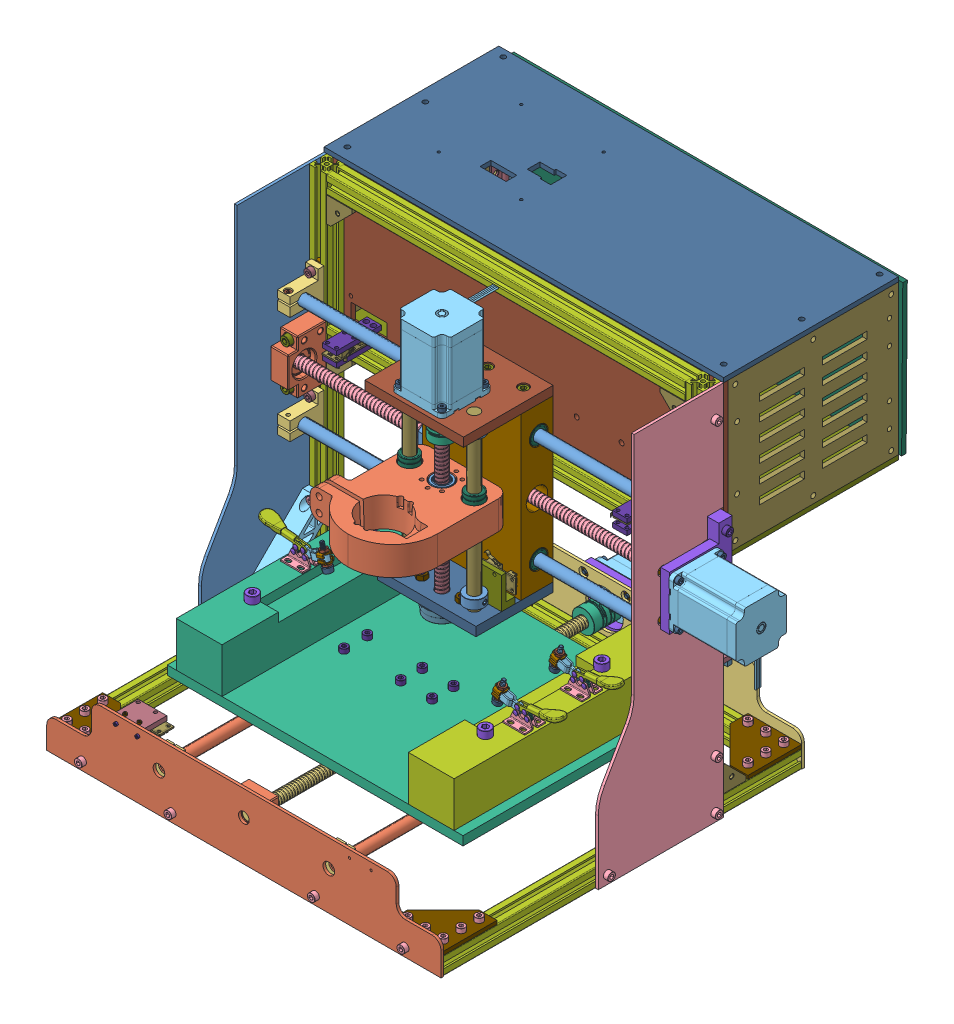
SolidWorks assembly CNC_DRILL1, configuration Default. Lengths in mm. (continued)
Components (placement in the parent): (continued)
- CUM_TAN_T-1: CUM_TAN_T [Default] at (66.2548 -100.7493 452.8517) x (-1 0 0) z (0 0 -1) size (20 34 34)
  - T-Nut_2020_M5.step-2-1: T-Nut_2020_M5.step-2 [Default] at (19.9061 6.5415 38.77) x (1 0 0) z (0 1 0) size (10 10.5 5)
  - T-Nut_2020_M5.step-2-2: T-Nut_2020_M5.step-2 [Default] at (19.9061 24.4415 20.87) size (10 10.5 5)
  - LBSBL6-2028-C_b-2-1: LBSBL6-2028-C_b-2 [Default] at (19.9061 8.5415 22.87) size (20 29.7 29.7)
- CUM_TAN_T-1-1: CUM_TAN_T-1 [Default] at (26.4425 -100.7493 427.1117) size (20 34 34)
  - T-Nut_2020_M5.step-2-1: T-Nut_2020_M5.step-2 [Default] at (19.9061 24.4415 20.87) size (10 10.5 5)
  - T-Nut_2020_M5.step-2-2: T-Nut_2020_M5.step-2 [Default] at (19.9061 6.5415 38.77) x (1 0 0) z (0 1 0) size (10 10.5 5)
  - LBSBL6-2028-C_b-2-1: LBSBL6-2028-C_b-2 [Default] at (19.9061 8.5415 22.87) size (20 29.7 29.7)
- CUM_TAN_T-2-1: CUM_TAN_T-2 [Default] at (486.2548 -100.7493 452.8517) x (-1 0 0) z (0 0 -1) size (20 34 34)
  - T-Nut_2020_M5.step-2-1: T-Nut_2020_M5.step-2 [Default] at (19.9061 24.4415 20.87) size (10 10.5 5)
  - T-Nut_2020_M5.step-2-2: T-Nut_2020_M5.step-2 [Default] at (19.9061 6.5415 38.77) x (1 0 0) z (0 1 0) size (10 10.5 5)
  - LBSBL6-2028-C_b-2-1: LBSBL6-2028-C_b-2 [Default] at (19.9061 8.5415 22.87) size (20 29.7 29.7)
- CUM_TAN_T-3-1: CUM_TAN_T-3 [Default] at (486.2548 -115.0778 441.4402) x (-1 0 0) z (0 1 0) size (20 34 34)
  - T-Nut_2020_M5.step-2-1: T-Nut_2020_M5.step-2 [Default] at (19.9061 24.4415 20.87) size (10 10.5 5)
  - T-Nut_2020_M5.step-2-2: T-Nut_2020_M5.step-2 [Default] at (19.9061 6.5415 38.77) x (1 0 0) z (0 1 0) size (10 10.5 5)
  - LBSBL6-2028-C_b-2-1: LBSBL6-2028-C_b-2 [Default] at (19.9061 8.5415 22.87) size (20 29.7 29.7)
- GH-201 (KECIL).STEP-1: GH-201 (KECIL).STEP [Default] at (384.0089 3.0167 494.044) size (81.05 32.54 23.05)
  - GH-201 (KECIL) PART 1.STEP-1: GH-201 (KECIL) PART 1.STEP [Default] at (0.3897 6.2755 23.667) size (24.52 11 10)
  - GH-201 (KECIL) PART 1.STEP-2: GH-201 (KECIL) PART 1.STEP [Default] at (24.8897 6.2755 0.6168) x (-1 0 0) z (0 0 -1) size (24.52 11 10)
  - GH-201 (KECIL) PART 2.STEP-1: GH-201 (KECIL) PART 2.STEP [Default] at (-14.4874 19.0399 16.1419) x (0.96092 -0.276826 0) z (0 0 1) size (28.48 12 8)
  - GH-201 (KECIL) PART 3.STEP-1: GH-201 (KECIL) PART 3.STEP [Default] at (16.2849 18.4306 12.167) x (0.434129 -0.900851 0) z (0 0 1) size (12 6 3)
  - GH-201 (KECIL) PART 4.STEP-1: GH-201 (KECIL) PART 4.STEP [Default] at (18.7026 25.6525 13.667) x (0.996652 0.081763 0) z (0 0 1) size (52.84 14.36 15)
  - GH-201 (KECIL) PIN.STEP-1: GH-201 (KECIL) PIN.STEP [Default] at (5.3978 13.1527 15.1668) x (0.991877 -0.127204 0) z (0 0 1) size (5 5 7.9)
  - GH-201 (KECIL) PIN.STEP-2: GH-201 (KECIL) PIN.STEP [Default] at (17.8978 13.1527 15.167) x (0.991877 -0.127204 0) z (0 0 1) size (5 5 7.9)
  - GH-201 (KECIL) PIN.STEP-3: GH-201 (KECIL) PIN.STEP [Default] at (7.1972 19.3987 15.1668) x (0.991877 -0.127204 0) z (0 0 1) size (5 5 7.9)
  - GH-201 (KECIL) PIN.STEP-4: GH-201 (KECIL) PIN.STEP [Default] at (15.2931 18.5578 15.1668) x (0.991877 -0.127204 0) z (0 0 1) size (5 5 7.9)
  - GH-201 (KECIL) CLIP.STEP-1: GH-201 (KECIL) CLIP.STEP [Default] at (-14.9027 17.5985 12.1419) x (-0.96092 0.276826 0) z (0 0 1) size (11 4 11)
  - GH-201 (KECIL) CLIP.STEP-2: GH-201 (KECIL) CLIP.STEP [Default] at (-12.1344 27.2077 12.1419) x (0.96092 -0.276826 0) z (0 0 1) size (11 4 11)
  - GH-201 (KECIL) PENEKAN.STEP-1: GH-201 (KECIL) PENEKAN.STEP [Default] at (-17.1675 9.7367 12.1419) x (0.942476 -0.271513 0.194986) z (-0.187366 0.053977 0.980806) size (10 27 10)
  - hex nut jam_am_B18.2.4.5M - Hex jam nut,  M5 x 0.8 --D-N.STEP-1: hex nut jam_am_B18.2.4.5M - Hex jam nut,  M5 x 0.8 --D-N.STEP [Default] at (-15.6501 15.0041 12.1419) x (0.96092 -0.276826 0) z (-0.276826 -0.96092 0) size (9.24 9.25 2.72)
  - hex nut jam_am_B18.2.4.5M - Hex jam nut,  M5 x 0.8 --D-N.STEP-2: hex nut jam_am_B18.2.4.5M - Hex jam nut,  M5 x 0.8 --D-N.STEP [Default] at (-11.387 29.8022 12.1419) x (0.96092 -0.276826 0) z (0.276826 0.96092 0) size (9.24 9.25 2.72)
- GH-201 (KECIL).STEP-1-1: GH-201 (KECIL).STEP-1 [Default] at (384.0089 3.0167 557.9937) size (81.05 32.54 23.05)
  - GH-201 (KECIL) PART 1.STEP-1: GH-201 (KECIL) PART 1.STEP [Default] at (24.8897 6.2755 0.6168) x (-1 0 0) z (0 0 -1) size (24.52 11 10)
  - GH-201 (KECIL) PART 1.STEP-2: GH-201 (KECIL) PART 1.STEP [Default] at (0.3897 6.2755 23.667) size (24.52 11 10)
  - GH-201 (KECIL) PART 2.STEP-1: GH-201 (KECIL) PART 2.STEP [Default] at (-14.4874 19.0399 16.1419) x (0.96092 -0.276826 0) z (0 0 1) size (28.48 12 8)
  - GH-201 (KECIL) PART 3.STEP-1: GH-201 (KECIL) PART 3.STEP [Default] at (16.2849 18.4306 12.167) x (0.434129 -0.900851 0) z (0 0 1) size (12 6 3)
  - GH-201 (KECIL) PART 4.STEP-1: GH-201 (KECIL) PART 4.STEP [Default] at (18.7026 25.6525 13.667) x (0.996652 0.081763 0) z (0 0 1) size (52.84 14.36 15)
  - GH-201 (KECIL) PIN.STEP-1: GH-201 (KECIL) PIN.STEP [Default] at (5.3978 13.1527 15.1668) x (0.991877 -0.127204 0) z (0 0 1) size (5 5 7.9)
  - GH-201 (KECIL) PIN.STEP-2: GH-201 (KECIL) PIN.STEP [Default] at (15.2931 18.5578 15.1668) x (0.991877 -0.127204 0) z (0 0 1) size (5 5 7.9)
  - GH-201 (KECIL) PIN.STEP-3: GH-201 (KECIL) PIN.STEP [Default] at (7.1972 19.3987 15.1668) x (0.991877 -0.127204 0) z (0 0 1) size (5 5 7.9)
  - GH-201 (KECIL) PIN.STEP-4: GH-201 (KECIL) PIN.STEP [Default] at (17.8978 13.1527 15.167) x (0.991877 -0.127204 0) z (0 0 1) size (5 5 7.9)
  - GH-201 (KECIL) CLIP.STEP-1: GH-201 (KECIL) CLIP.STEP [Default] at (-14.9027 17.5985 12.1419) x (-0.96092 0.276826 0) z (0 0 1) size (11 4 11)
  - GH-201 (KECIL) CLIP.STEP-2: GH-201 (KECIL) CLIP.STEP [Default] at (-12.1344 27.2077 12.1419) x (0.96092 -0.276826 0) z (0 0 1) size (11 4 11)
  - GH-201 (KECIL) PENEKAN.STEP-1: GH-201 (KECIL) PENEKAN.STEP [Default] at (-17.1675 9.7367 12.1419) x (0.942476 -0.271513 0.194986) z (-0.187366 0.053977 0.980806) size (10 27 10)
  - hex nut jam_am_B18.2.4.5M - Hex jam nut,  M5 x 0.8 --D-N.STEP-1: hex nut jam_am_B18.2.4.5M - Hex jam nut,  M5 x 0.8 --D-N.STEP [Default] at (-15.6501 15.0041 12.1419) x (0.96092 -0.276826 0) z (-0.276826 -0.96092 0) size (9.24 9.25 2.72)
  - hex nut jam_am_B18.2.4.5M - Hex jam nut,  M5 x 0.8 --D-N.STEP-2: hex nut jam_am_B18.2.4.5M - Hex jam nut,  M5 x 0.8 --D-N.STEP [Default] at (-11.387 29.8022 12.1419) x (0.96092 -0.276826 0) z (0.276826 0.96092 0) size (9.24 9.25 2.72)
- GH-201 (KECIL).STEP-2-1: GH-201 (KECIL).STEP-2 [Default] at (129.1884 3.0167 550.2775) x (-1 0 0) z (0 0 -1) size (81.05 32.54 23.05)
  - GH-201 (KECIL) PART 1.STEP-1: GH-201 (KECIL) PART 1.STEP [Default] at (0.3897 6.2755 23.667) size (24.52 11 10)
  - GH-201 (KECIL) PART 1.STEP-2: GH-201 (KECIL) PART 1.STEP [Default] at (24.8897 6.2755 0.6168) x (-1 0 0) z (0 0 -1) size (24.52 11 10)
  - GH-201 (KECIL) PART 2.STEP-1: GH-201 (KECIL) PART 2.STEP [Default] at (-14.4874 19.0399 16.1419) x (0.96092 -0.276826 0) z (0 0 1) size (28.48 12 8)
  - GH-201 (KECIL) PART 3.STEP-1: GH-201 (KECIL) PART 3.STEP [Default] at (16.2849 18.4306 12.167) x (0.434129 -0.900851 0) z (0 0 1) size (12 6 3)
  - GH-201 (KECIL) PART 4.STEP-1: GH-201 (KECIL) PART 4.STEP [Default] at (18.7026 25.6525 13.667) x (0.996652 0.081763 0) z (0 0 1) size (52.84 14.36 15)
  - GH-201 (KECIL) PIN.STEP-1: GH-201 (KECIL) PIN.STEP [Default] at (7.1972 19.3987 15.1668) x (0.991877 -0.127204 0) z (0 0 1) size (5 5 7.9)
  - GH-201 (KECIL) PIN.STEP-2: GH-201 (KECIL) PIN.STEP [Default] at (5.3978 13.1527 15.1668) x (0.991877 -0.127204 0) z (0 0 1) size (5 5 7.9)
  - GH-201 (KECIL) PIN.STEP-3: GH-201 (KECIL) PIN.STEP [Default] at (17.8978 13.1527 15.167) x (0.991877 -0.127204 0) z (0 0 1) size (5 5 7.9)
  - GH-201 (KECIL) PIN.STEP-4: GH-201 (KECIL) PIN.STEP [Default] at (15.2931 18.5578 15.1668) x (0.991877 -0.127204 0) z (0 0 1) size (5 5 7.9)
  - GH-201 (KECIL) CLIP.STEP-1: GH-201 (KECIL) CLIP.STEP [Default] at (-14.9027 17.5985 12.1419) x (-0.96092 0.276826 0) z (0 0 1) size (11 4 11)
  - GH-201 (KECIL) CLIP.STEP-2: GH-201 (KECIL) CLIP.STEP [Default] at (-12.1344 27.2077 12.1419) x (0.96092 -0.276826 0) z (0 0 1) size (11 4 11)
  - GH-201 (KECIL) PENEKAN.STEP-1: GH-201 (KECIL) PENEKAN.STEP [Default] at (-17.1675 9.7367 12.1419) x (0.942476 -0.271513 0.194986) z (-0.187366 0.053977 0.980806) size (10 27 10)
  - hex nut jam_am_B18.2.4.5M - Hex jam nut,  M5 x 0.8 --D-N.STEP-1: hex nut jam_am_B18.2.4.5M - Hex jam nut,  M5 x 0.8 --D-N.STEP [Default] at (-11.387 29.8022 12.1419) x (0.96092 -0.276826 0) z (0.276826 0.96092 0) size (9.24 9.25 2.72)
  - hex nut jam_am_B18.2.4.5M - Hex jam nut,  M5 x 0.8 --D-N.STEP-2: hex nut jam_am_B18.2.4.5M - Hex jam nut,  M5 x 0.8 --D-N.STEP [Default] at (-15.6501 15.0041 12.1419) x (0.96092 -0.276826 0) z (-0.276826 -0.96092 0) size (9.24 9.25 2.72)
- Assem1-1: Assem1 [Default] at (138.0975 -49.2059 785.2437) x (-1 0 0) z (0 0 -1) size (40.5 13.14 31.22)
  - Limit_switch-1: Limit_switch [Default] at (6.9988 2.8611 61.862) x (-1 0 0) z (0 0 -1) size (40.5 9 22.67)
  - Part101-1: Part101 [Default] at (11.2488 9.4981 60.262) x (1 0 0) z (0 -1 0) size (32 25 5)
  - Part15-1: Part15 [Default] at (11.2488 1.9981 45.262) size (32 5 5)
- Assem1-1-1: Assem1-1 [Default] at (371.0998 -49.2059 294.7198) size (40.5 13.14 31.22)
  - Limit_switch-1: Limit_switch [Default] at (6.9988 2.8611 61.862) x (-1 0 0) z (0 0 -1) size (40.5 9 22.67)
  - Part101-1: Part101 [Default] at (11.2488 9.4981 60.262) x (1 0 0) z (0 -1 0) size (32 25 5)
  - Part15-1: Part15 [Default] at (11.2488 1.9981 45.262) size (32 5 5)
- CONG_TAC_2-1: CONG_TAC_2 [Default] at (248.0157 229.2239 470.9282) x (-1 0 0) z (0 0 1) size (42.3 46.22 15)
  - Limit_switch-1: Limit_switch [Default] at (24.7058 33.7317 35.7236) x (1 0 0) z (0 -1 0) size (40.5 9 22.67)
  - 3D_IN_2-1: 3D_IN_2 [Default] at (18.6558 32.1317 36.4836) size (32 40 15)
- CONG_TAC_3-1: CONG_TAC_3 [Default] at (285.9024 40.7719 478.8031) size (42.3 41.22 15)
  - Limit_switch-1: Limit_switch [Default] at (20.0775 32.9203 29.9187) x (1 0 0) z (0 -1 0) size (40.5 9 22.67)
  - 3D_IN_3-1: 3D_IN_3 [Default] at (14.0275 31.3203 30.6787) size (32 35 15)
- Assem21-1: Assem21 [Default] at (134.1207 169.7573 469.2393) x (0 0 -1) z (-1 0 0) size (50.1 16.81 22.67)
  - Limit_switch-1: Limit_switch [Default] at (4.4076 3.2051 40.1721) size (40.5 9 22.67)
  - Part178-1: Part178 [Default] at (9.2576 3.9651 39.7721) size (50 5 16)
  - Part178-2: Part178 [Default] at (9.2576 -7.8449 39.7721) size (50 5 16)
- Assem21-1-1: Assem21-1 [Default] at (378.5766 168.6371 469.2393) x (0 0 -1) z (1 0 0) size (50.1 16.81 22.67)
  - Limit_switch-1: Limit_switch [Default] at (4.4076 3.2051 40.1721) size (40.5 9 22.67)
  - Part178-1: Part178 [Default] at (9.2576 3.9651 39.7721) size (50 5 16)
  - Part178-2: Part178 [Default] at (9.2576 -7.8449 39.7721) size (50 5 16)
- socket head cap screw_iso(ISO 4762 M5 x 8 - 8N)-1: socket head cap screw_iso(ISO 4762 M5 x 8 - 8N) [Default] at (66.3487 -83.2078 729.9817) x (0 -1 0) z (0 0 1) size (13 8.5 8.5)
- socket head cap screw_iso(ISO 4762 M5 x 8 - 8N)-2: socket head cap screw_iso(ISO 4762 M5 x 8 - 8N) [Default] at (446.3487 -83.2078 349.9817) x (0 -1 0) z (0 0 1) size (13 8.5 8.5)
- socket head cap screw_iso(ISO 4762 M5 x 8 - 8N)-3: socket head cap screw_iso(ISO 4762 M5 x 8 - 8N) [Default] at (46.3487 -83.2078 689.9817) x (0 -1 0) z (0 0 1) size (13 8.5 8.5)
- socket head cap screw_iso(ISO 4762 M5 x 8 - 8N)-4: socket head cap screw_iso(ISO 4762 M5 x 8 - 8N) [Default] at (46.3487 -83.2078 729.9817) x (0 -1 0) z (0 0 1) size (13 8.5 8.5)
- socket head cap screw_iso(ISO 4762 M5 x 8 - 8N)-5: socket head cap screw_iso(ISO 4762 M5 x 8 - 8N) [Default] at (28.3487 -102.2078 559.9817) size (13 8.5 8.5)
- socket head cap screw_iso(ISO 4762 M5 x 8 - 8N)-6: socket head cap screw_iso(ISO 4762 M5 x 8 - 8N) [Default] at (46.3487 -8.7078 458.9817) x (0 0 -1) z (1 0 0) size (13 8.5 8.5)
- socket head cap screw_iso(ISO 4762 M5 x 8 - 8N)-7: socket head cap screw_iso(ISO 4762 M5 x 8 - 8N) [Default] at (466.3487 -83.2078 729.9817) x (0 -1 0) z (0 0 1) size (13 8.5 8.5)
- socket head cap screw_iso(ISO 4762 M5 x 8 - 8N)-8: socket head cap screw_iso(ISO 4762 M5 x 8 - 8N) [Default] at (447.3487 -102.2078 439.9817) size (13 8.5 8.5)
- socket head cap screw_iso(ISO 4762 M5 x 8 - 8N)-9: socket head cap screw_iso(ISO 4762 M5 x 8 - 8N) [Default] at (466.3487 -83.2078 709.9817) x (0 -1 0) z (0 0 1) size (13 8.5 8.5)
- socket head cap screw_iso(ISO 4762 M5 x 8 - 8N)-10: socket head cap screw_iso(ISO 4762 M5 x 8 - 8N) [Default] at (336.3487 -102.2078 331.9817) x (0 0 1) z (-1 0 0) size (13 8.5 8.5)
- socket head cap screw_iso(ISO 4762 M5 x 8 - 8N)-11: socket head cap screw_iso(ISO 4762 M5 x 8 - 8N) [Default] at (65.3487 -62.2078 439.9817) x (-1 0 0) z (0 0.924225 0.381849) size (13 8.5 8.5)
- socket head cap screw_iso(ISO 4762 M5 x 8 - 8N)-12: socket head cap screw_iso(ISO 4762 M5 x 8 - 8N) [Default] at (466.3487 -83.2078 533.4817) x (0 -1 0) z (0 0 1) size (13 8.5 8.5)
- socket head cap screw_iso(ISO 4762 M5 x 8 - 8N)-13: socket head cap screw_iso(ISO 4762 M5 x 8 - 8N) [Default] at (436.8487 -102.2078 747.9817) x (0 0 -1) z (1 0 0) size (13 8.5 8.5)
- socket head cap screw_iso(ISO 4762 M5 x 8 - 8N)-14: socket head cap screw_iso(ISO 4762 M5 x 8 - 8N) [Default] at (46.3487 -83.2078 465.8817) x (0 -1 0) z (0.924225 0 -0.381849) size (13 8.5 8.5)
- socket head cap screw_iso(ISO 4762 M5 x 8 - 8N)-15: socket head cap screw_iso(ISO 4762 M5 x 8 - 8N) [Default] at (466.3487 -83.2078 369.9817) x (0 -1 0) z (0 0 1) size (13 8.5 8.5)
- socket head cap screw_iso(ISO 4762 M5 x 8 - 8N)-16: socket head cap screw_iso(ISO 4762 M5 x 8 - 8N) [Default] at (46.3487 -76.3078 458.9817) x (0 0 -1) z (0.381849 -0.924225 0) size (13 8.5 8.5)
- socket head cap screw_iso(ISO 4762 M5 x 8 - 8N)-17: socket head cap screw_iso(ISO 4762 M5 x 8 - 8N) [Default] at (484.3487 -47.2078 439.9817) x (-1 0 0) z (0 0.924225 0.381849) size (13 8.5 8.5)
- socket head cap screw_iso(ISO 4762 M5 x 8 - 8N)-18: socket head cap screw_iso(ISO 4762 M5 x 8 - 8N) [Default] at (176.3487 -102.2078 331.9817) x (0 0 1) z (-1 0 0) size (13 8.5 8.5)
- socket head cap screw_iso(ISO 4762 M5 x 8 - 8N)-19: socket head cap screw_iso(ISO 4762 M5 x 8 - 8N) [Default] at (466.3487 -83.2078 465.8817) x (0 -1 0) z (0.913871 0 -0.406005) size (13 8.5 8.5)
- socket head cap screw_iso(ISO 4762 M5 x 8 - 8N)-20: socket head cap screw_iso(ISO 4762 M5 x 8 - 8N) [Default] at (28.3487 77.7922 439.9817) size (13 8.5 8.5)
- socket head cap screw_iso(ISO 4762 M5 x 8 - 8N)-21: socket head cap screw_iso(ISO 4762 M5 x 8 - 8N) [Default] at (46.3487 -83.2078 414.0817) x (0 -1 0) z (0 0 1) size (13 8.5 8.5)
- socket head cap screw_iso(ISO 4762 M5 x 8 - 8N)-22: socket head cap screw_iso(ISO 4762 M5 x 8 - 8N) [Default] at (76.8487 -102.2078 747.9817) x (0 0 -1) z (1 0 0) size (13 8.5 8.5)
- socket head cap screw_iso(ISO 4762 M5 x 8 - 8N)-23: socket head cap screw_iso(ISO 4762 M5 x 8 - 8N) [Default] at (176.8487 -102.2078 747.9817) x (0 0 -1) z (1 0 0) size (13 8.5 8.5)
- socket head cap screw_iso(ISO 4762 M5 x 8 - 8N)-24: socket head cap screw_iso(ISO 4762 M5 x 8 - 8N) [Default] at (76.3487 -102.2078 331.9817) x (0 0 1) z (-1 0 0) size (13 8.5 8.5)
- socket head cap screw_iso(ISO 4762 M5 x 8 - 8N)-25: socket head cap screw_iso(ISO 4762 M5 x 8 - 8N) [Default] at (447.3487 -82.2078 439.9817) size (13 8.5 8.5)
- socket head cap screw_iso(ISO 4762 M5 x 8 - 8N)-26: socket head cap screw_iso(ISO 4762 M5 x 8 - 8N) [Default] at (65.3487 -82.2078 439.9817) x (-1 0 0) z (0 0.924225 0.381849) size (13 8.5 8.5)
- socket head cap screw_iso(ISO 4762 M5 x 8 - 8N)-27: socket head cap screw_iso(ISO 4762 M5 x 8 - 8N) [Default] at (446.3487 -83.2078 729.9817) x (0 -1 0) z (0 0 1) size (13 8.5 8.5)
- socket head cap screw_iso(ISO 4762 M5 x 8 - 8N)-28: socket head cap screw_iso(ISO 4762 M5 x 8 - 8N) [Default] at (447.3487 -102.2078 479.9817) size (13 8.5 8.5)
- socket head cap screw_iso(ISO 4762 M5 x 8 - 8N)-29: socket head cap screw_iso(ISO 4762 M5 x 8 - 8N) [Default] at (466.3487 -83.2078 689.9817) x (0 -1 0) z (0 0 1) size (13 8.5 8.5)
- socket head cap screw_iso(ISO 4762 M5 x 8 - 8N)-30: socket head cap screw_iso(ISO 4762 M5 x 8 - 8N) [Default] at (65.3487 -102.2078 459.9817) x (-1 0 0) z (0 0.924225 0.381849) size (13 8.5 8.5)
- socket head cap screw_iso(ISO 4762 M5 x 8 - 8N)-31: socket head cap screw_iso(ISO 4762 M5 x 8 - 8N) [Default] at (46.3487 -76.3078 420.9817) x (0 0 1) z (-0.565374 -0.824835 0) size (13 8.5 8.5)
- socket head cap screw_iso(ISO 4762 M5 x 8 - 8N)-32: socket head cap screw_iso(ISO 4762 M5 x 8 - 8N) [Default] at (466.3487 -83.2078 349.9817) x (0 -1 0) z (0 0 1) size (13 8.5 8.5)
- socket head cap screw_iso(ISO 4762 M5 x 8 - 8N)-33: socket head cap screw_iso(ISO 4762 M5 x 8 - 8N) [Default] at (65.3487 -102.2078 439.9817) x (-1 0 0) z (0 0.924225 0.381849) size (13 8.5 8.5)
- socket head cap screw_iso(ISO 4762 M5 x 8 - 8N)-34: socket head cap screw_iso(ISO 4762 M5 x 8 - 8N) [Default] at (466.3487 -83.2078 389.9817) x (0 -1 0) z (0 0 1) size (13 8.5 8.5)
- socket head cap screw_iso(ISO 4762 M5 x 8 - 8N)-35: socket head cap screw_iso(ISO 4762 M5 x 8 - 8N) [Default] at (484.3487 77.7922 439.9817) x (-1 0 0) z (0 0.924225 0.381849) size (13 8.5 8.5)
- socket head cap screw_iso(ISO 4762 M5 x 8 - 8N)-36: socket head cap screw_iso(ISO 4762 M5 x 8 - 8N) [Default] at (46.3487 -83.2078 533.4817) x (0 -1 0) z (0 0 1) size (13 8.5 8.5)
- socket head cap screw_iso(ISO 4762 M5 x 8 - 8N)-37: socket head cap screw_iso(ISO 4762 M5 x 8 - 8N) [Default] at (28.3487 -47.2078 439.9817) size (13 8.5 8.5)
- socket head cap screw_iso(ISO 4762 M5 x 8 - 8N)-38: socket head cap screw_iso(ISO 4762 M5 x 8 - 8N) [Default] at (66.3487 -83.2078 349.9817) x (0 -1 0) z (0 0 1) size (13 8.5 8.5)
- socket head cap screw_iso(ISO 4762 M5 x 8 - 8N)-39: socket head cap screw_iso(ISO 4762 M5 x 8 - 8N) [Default] at (426.3487 -83.2078 349.9817) x (0 -1 0) z (0 0 1) size (13 8.5 8.5)
- socket head cap screw_iso(ISO 4762 M5 x 8 - 8N)-40: socket head cap screw_iso(ISO 4762 M5 x 8 - 8N) [Default] at (86.3487 -83.2078 349.9817) x (0 -1 0) z (0 0 1) size (13 8.5 8.5)
- socket head cap screw_iso(ISO 4762 M5 x 8 - 8N)-41: socket head cap screw_iso(ISO 4762 M5 x 8 - 8N) [Default] at (46.3487 -83.2078 349.9817) x (0 -1 0) z (0 0 1) size (13 8.5 8.5)
- socket head cap screw_iso(ISO 4762 M5 x 8 - 8N)-42: socket head cap screw_iso(ISO 4762 M5 x 8 - 8N) [Default] at (426.3487 -83.2078 729.9817) x (0 -1 0) z (0 0 1) size (13 8.5 8.5)
- socket head cap screw_iso(ISO 4762 M5 x 8 - 8N)-43: socket head cap screw_iso(ISO 4762 M5 x 8 - 8N) [Default] at (28.3487 -102.2078 439.9817) size (13 8.5 8.5)
- socket head cap screw_iso(ISO 4762 M5 x 8 - 8N)-44: socket head cap screw_iso(ISO 4762 M5 x 8 - 8N) [Default] at (466.3487 -76.3078 458.9817) x (0 0 -1) z (0.994603 0.103758 0) size (13 8.5 8.5)
- socket head cap screw_iso(ISO 4762 M5 x 8 - 8N)-45: socket head cap screw_iso(ISO 4762 M5 x 8 - 8N) [Default] at (466.3487 -8.7078 458.9817) x (0 0 -1) z (1 0 0) size (13 8.5 8.5)
- socket head cap screw_iso(ISO 4762 M5 x 8 - 8N)-46: socket head cap screw_iso(ISO 4762 M5 x 8 - 8N) [Default] at (484.3487 -102.2078 439.9817) x (-1 0 0) z (0 0.924225 0.381849) size (13 8.5 8.5)
- socket head cap screw_iso(ISO 4762 M5 x 8 - 8N)-47: socket head cap screw_iso(ISO 4762 M5 x 8 - 8N) [Default] at (336.8487 -102.2078 747.9817) x (0 0 -1) z (1 0 0) size (13 8.5 8.5)
- socket head cap screw_iso(ISO 4762 M5 x 8 - 8N)-48: socket head cap screw_iso(ISO 4762 M5 x 8 - 8N) [Default] at (46.3487 -83.2078 709.9817) x (0 -1 0) z (0 0 1) size (13 8.5 8.5)
- socket head cap screw_iso(ISO 4762 M5 x 8 - 8N)-49: socket head cap screw_iso(ISO 4762 M5 x 8 - 8N) [Default] at (86.3487 -83.2078 729.9817) x (0 -1 0) z (0 0 1) size (13 8.5 8.5)
- socket head cap screw_iso(ISO 4762 M5 x 8 - 8N)-50: socket head cap screw_iso(ISO 4762 M5 x 8 - 8N) [Default] at (447.3487 -62.2078 439.9817) size (13 8.5 8.5)
- socket head cap screw_iso(ISO 4762 M5 x 8 - 8N)-51: socket head cap screw_iso(ISO 4762 M5 x 8 - 8N) [Default] at (436.3487 -102.2078 331.9817) x (0 0 1) z (-1 0 0) size (13 8.5 8.5)
- socket head cap screw_iso(ISO 4762 M5 x 8 - 8N)-52: socket head cap screw_iso(ISO 4762 M5 x 8 - 8N) [Default] at (484.3487 277.7922 439.9817) x (-1 0 0) z (0 0.924225 0.381849) size (13 8.5 8.5)
- socket head cap screw_iso(ISO 4762 M5 x 8 - 8N)-53: socket head cap screw_iso(ISO 4762 M5 x 8 - 8N) [Default] at (484.3487 -102.2078 559.9817) x (-1 0 0) z (0 0.924225 0.381849) size (13 8.5 8.5)
- socket head cap screw_iso(ISO 4762 M5 x 8 - 8N)-54: socket head cap screw_iso(ISO 4762 M5 x 8 - 8N) [Default] at (466.3487 -83.2078 414.0817) x (0 -1 0) z (-0.997969 0 -0.063694) size (13 8.5 8.5)
- socket head cap screw_iso(ISO 4762 M5 x 8 - 8N)-55: socket head cap screw_iso(ISO 4762 M5 x 8 - 8N) [Default] at (65.3487 -102.2078 479.9817) x (-1 0 0) z (0 0.924225 0.381849) size (13 8.5 8.5)
- socket head cap screw_iso(ISO 4762 M5 x 8 - 8N)-56: socket head cap screw_iso(ISO 4762 M5 x 8 - 8N) [Default] at (28.3487 277.7922 439.9817) size (13 8.5 8.5)
- socket head cap screw_iso(ISO 4762 M5 x 8 - 8N)-57: socket head cap screw_iso(ISO 4762 M5 x 8 - 8N) [Default] at (46.3487 -83.2078 389.9817) x (0 -1 0) z (0 0 1) size (13 8.5 8.5)
- socket head cap screw_iso(ISO 4762 M5 x 8 - 8N)-58: socket head cap screw_iso(ISO 4762 M5 x 8 - 8N) [Default] at (46.3487 -83.2078 369.9817) x (0 -1 0) z (0 0 1) size (13 8.5 8.5)
- socket head cap screw_iso(ISO 4762 M5 x 8 - 8N)-59: socket head cap screw_iso(ISO 4762 M5 x 8 - 8N) [Default] at (447.3487 -102.2078 459.9817) size (13 8.5 8.5)
- socket head cap screw_iso(ISO 4762 M5 x 8 - 8N)-60: socket head cap screw_iso(ISO 4762 M5 x 8 - 8N) [Default] at (466.3487 -76.3078 420.9817) x (0 0 1) z (0.712194 0.701982 0) size (13 8.5 8.5)
- KE_GOC_2020-1: KE_GOC_2020 [Default] at (56.3487 -82.2078 459.9817) x (0 1 0) z (0 0 -1) size (60 4 60)
- KE_GOC_2020-2: KE_GOC_2020 [Default] at (452.3487 -82.2078 459.9817) x (0 1 0) z (0 0 -1) size (60 4 60)
- KE_GOC_2020-3: KE_GOC_2020 [Default] at (66.3487 -92.2078 709.9817) size (60 4 60)
- KE_GOC_2020-4: KE_GOC_2020 [Default] at (446.3487 -92.2078 709.9817) x (0 0 -1) z (1 0 0) size (60 4 60)
- KE_GOC_2020-5: KE_GOC_2020 [Default] at (66.3487 -92.2078 369.9817) x (0 0 1) z (-1 0 0) size (60 4 60)
- KE_GOC_2020-6: KE_GOC_2020 [Default] at (446.3487 -88.2078 369.9817) x (0 0 1) z (1 0 0) size (60 4 60)
- 111113t-1-1: 111113t-1 [Default] at (75.7784 180.7512 355.7133) x (0 0 1) z (0 -1 0) size (140 3 420)
- Part123333333-1: Part123333333 [Default] at (256.8487 -67.2078 739.9817) x (-1 0 0) z (0 0 1) size (440 73 3)
- Part123333333 - 2-1: Part123333333 - 2 [Default] at (256.3487 -67.2078 336.9817) x (-1 0 0) z (0 0 1) size (440 77 3)
- qqsedvcgdsxfdxdbdxggb-1-1: qqsedvcgdsxfdxdbdxggb-1 [Default] at (518.7784 180.7512 355.7133) x (0 0 1) z (0 -1 0) size (140 3 420)
- Part46-1: Part46 [Default] at (56.3487 -51.4446 490.7449) x (0 -0.707107 0.707107) z (0 -0.707107 -0.707107) size (127.28 20 20)
- Part46-2: Part46 [Default] at (476.3487 -51.4446 490.7449) x (0 -0.707107 0.707107) z (0 -0.707107 -0.707107) size (127.28 20 20)
- 455_1-1: 455_1 [Default] at (101.5987 -17.2078 538.1607) x (0 0 1) z (0 1 0) size (250 51 50)
- 455-1: 455 [Default] at (411.5987 -17.2078 538.1607) x (0 0 -1) z (0 1 0) size (250 51 50)
- socket head cap screw_iso(ISO 4762 M8 x 65 - 28N)-1: socket head cap screw_iso(ISO 4762 M8 x 65 - 28N) [Default] at (386.5987 15.7922 473.1607) x (0 -1 0) z (0 0 1) size (73 13 13)
- socket head cap screw_iso(ISO 4762 M8 x 65 - 28N)-2: socket head cap screw_iso(ISO 4762 M8 x 65 - 28N) [Default] at (386.5987 15.7922 603.1607) x (0 -1 0) z (0 0 1) size (73 13 13)
- socket head cap screw_iso(ISO 4762 M8 x 65 - 28N)-3: socket head cap screw_iso(ISO 4762 M8 x 65 - 28N) [Default] at (126.5987 15.7922 603.1607) x (0 -1 0) z (0 0 1) size (73 13 13)
- socket head cap screw_iso(ISO 4762 M8 x 65 - 28N)-4: socket head cap screw_iso(ISO 4762 M8 x 65 - 28N) [Default] at (126.5987 15.7922 473.1607) x (0 -1 0) z (0 0 1) size (73 13 13)
- hex nut style 1 gradeab_iso(ISO - 4032 - M8 - W - N)-1: hex nut style 1 gradeab_iso(ISO - 4032 - M8 - W - N) [Default] at (126.5987 -59.0078 473.1607) x (1 0 0) z (0 -1 0) size (13 15.01 6.8)
- hex nut style 1 gradeab_iso(ISO - 4032 - M8 - W - N)-2: hex nut style 1 gradeab_iso(ISO - 4032 - M8 - W - N) [Default] at (126.5987 -59.0078 603.1607) x (1 0 0) z (0 -1 0) size (13 15.01 6.8)
- hex nut style 1 gradeab_iso(ISO - 4032 - M8 - W - N)-3: hex nut style 1 gradeab_iso(ISO - 4032 - M8 - W - N) [Default] at (386.5987 -59.0078 473.1607) x (1 0 0) z (0 -1 0) size (13 15.01 6.8)
- hex nut style 1 gradeab_iso(ISO - 4032 - M8 - W - N)-4: hex nut style 1 gradeab_iso(ISO - 4032 - M8 - W - N) [Default] at (386.5987 -59.0078 603.1607) x (1 0 0) z (0 -1 0) size (13 15.01 6.8)
- NAP_TREN-1: NAP_TREN [Default] at (256.3487 307.7922 332.4817) size (446 5 195)
- Part54Z-1: Part54Z [Default] at (258.3487 232.7922 424.9817) size (446 167 5)
- Part54Z(3)_1-1: Part54Z(3)_1 [Default] at (38.3487 224.2922 329.9817) x (0 0 1) z (-1 0 0) size (190 167 5)
- Part54Z(3)_1-2: Part54Z(3)_1 [Default] at (479.3487 224.2922 329.9817) x (0 0 1) z (-1 0 0) size (190 167 5)
- Part4-1: Part4 [Default] at (40.3487 184.3021 246.2201) x (0 -0.007716 -0.99997) z (1 0 0) size (18 50 6)
- Part4-2: Part4 [Default] at (40.3487 264.3021 246.2201) x (0 -0.007716 -0.99997) z (1 0 0) size (18 50 6)
- Part3-1: Part3 [Default] at (48.8507 264.2125 234.6013) x (0.999998 0.000016 0.002014) z (-0.002014 0.007716 0.999968) size (18 50 6)
- Part3-2: Part3 [Default] at (48.8507 184.2125 234.6013) x (0.999998 0.000016 0.002014) z (-0.002014 0.007716 0.999968) size (18 50 6)
- Part2-1: Part2 [Default] at (262.3643 224.163 228.3402) x (0.999998 0.000016 0.002014) z (0 -0.99997 0.007716) size (440 5 167)
- Part198-1: Part198 [Default] at (256.3487 135.7922 332.4817) size (446 5 195)
- socket head cap screw_iso(ISO 4762 M2 x 10 - 10N)-1: socket head cap screw_iso(ISO 4762 M2 x 10 - 10N) [Default] at (138.8487 -47.2078 744.9817) x (0 0 -1) z (1 0 0) size (12 3.8 3.8)
- socket head cap screw_iso(ISO 4762 M2 x 10 - 10N)-2: socket head cap screw_iso(ISO 4762 M2 x 10 - 10N) [Default] at (114.8487 -47.2078 744.9817) x (0 0 -1) z (1 0 0) size (12 3.8 3.8)
- socket head cap screw_iso(ISO 4762 M2 x 10 - 10N)-3: socket head cap screw_iso(ISO 4762 M2 x 10 - 10N) [Default] at (370.3487 -47.2078 334.9817) x (0 0 1) z (-1 0 0) size (12 3.8 3.8)
- socket head cap screw_iso(ISO 4762 M2 x 10 - 10N)-4: socket head cap screw_iso(ISO 4762 M2 x 10 - 10N) [Default] at (394.3487 -47.2078 334.9817) x (0 0 1) z (-1 0 0) size (12 3.8 3.8)
- socket head cap screw_iso(ISO 4762 M2 x 12 - 12N)-1: socket head cap screw_iso(ISO 4762 M2 x 12 - 12N) [Default] at (390.3487 -37.7078 342.4817) x (0 -1 0) z (0 0 1) size (14 3.8 3.8)
- socket head cap screw_iso(ISO 4762 M2 x 12 - 12N)-2: socket head cap screw_iso(ISO 4762 M2 x 12 - 12N) [Default] at (134.8487 -37.7078 737.4817) x (0 -1 0) z (0 0 1) size (14 3.8 3.8)
- socket head cap screw_iso(ISO 4762 M2 x 12 - 12N)-3: socket head cap screw_iso(ISO 4762 M2 x 12 - 12N) [Default] at (374.3487 -37.7078 342.4817) x (0 -1 0) z (0 0 1) size (14 3.8 3.8)
- socket head cap screw_iso(ISO 4762 M2 x 12 - 12N)-4: socket head cap screw_iso(ISO 4762 M2 x 12 - 12N) [Default] at (118.8487 -37.7078 737.4817) x (0 -1 0) z (0 0 1) size (14 3.8 3.8)
